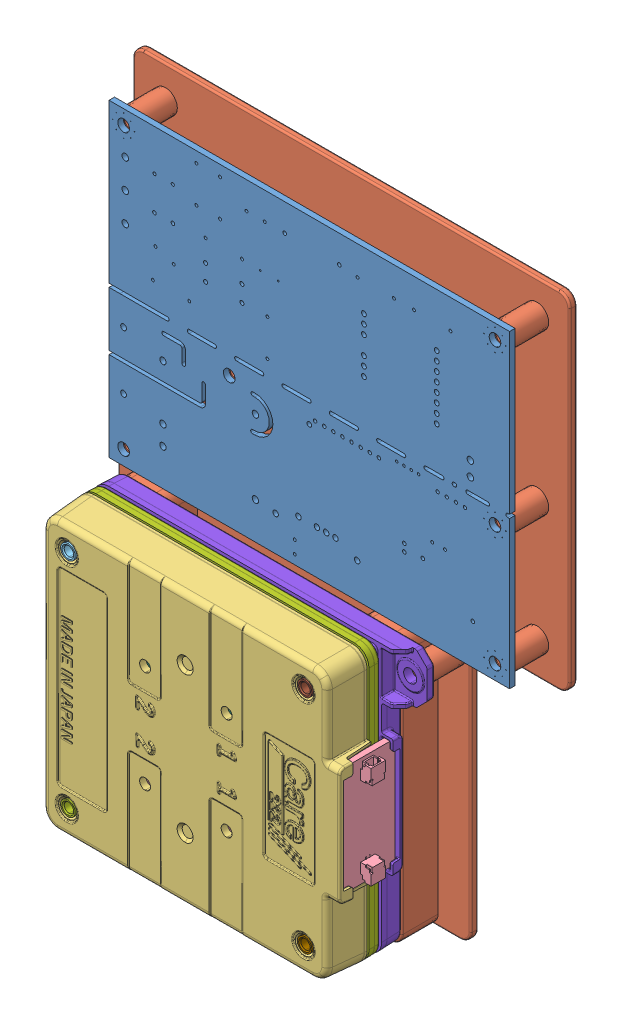
SolidWorks assembly osluv_test_assembly, configuration Default. Lengths in mm.
Overall size (124.12 167.88 32.3).
38 component instances, 33 part files, 8 mates.
Components (placement in the parent):
- osluv_pcb-1: osluv_pcb [Default] at (-161.3043 106.25 19.6144) size (110 85 1.51)
- test_fixture-1: test_fixture [Default] at (-161.3043 106.25 19.6144) x (-1 0 0) z (0 0 -1) size (124.12 167.88 12)
- emitter-1: emitter [Default] at (-120.388 -50.4736 -52.2117) x (0 -1 0) z (0 0 1) size (75 97 26.91)
  - emitter.step-1: emitter.step [Default] at origin size (75 97 26.91)
    - DRW1103739_UXFL70-222B4-UIA-Z1.STEP.step-1: DRW1103739_UXFL70-222B4-UIA-Z1.STEP.step [Default] at (-18.8418 87.9656 71.8261) size (75 97 26.91)
      - Z01_DRW1103184_LampCaseA.STEP.step-1: Z01_DRW1103184_LampCaseA.STEP.step [Default] at (0 3.0667 9.49) x (1 0 0) z (0 -1 0) size (75 10.8 82.07)
        - Z01_DRW1103184_LampCaseA-Part-1.STEP.step-1: Z01_DRW1103184_LampCaseA-Part-1.STEP.step [Default] at origin size (75 10.8 82.07)
        - Z01_DRW1103184_LampCaseA-Part-2.STEP.step-1: Z01_DRW1103184_LampCaseA-Part-2.STEP.step [Default] at origin size (4.3 4 4.3)
        - Z01_DRW1103184_LampCaseA-Part-3.STEP.step-1: Z01_DRW1103184_LampCaseA-Part-3.STEP.step [Default] at origin size (4.3 4 4.3)
        - Z01_DRW1103184_LampCaseA-Part-4.STEP.step-1: Z01_DRW1103184_LampCaseA-Part-4.STEP.step [Default] at origin size (4.3 4 4.3)
        - Z01_DRW1103184_LampCaseA-Part-5.STEP.step-1: Z01_DRW1103184_LampCaseA-Part-5.STEP.step [Default] at origin size (4.3 4 4.3)
        - Z01_DRW1103184_LampCaseA-Part-6.STEP.step-1: Z01_DRW1103184_LampCaseA-Part-6.STEP.step [Default] at origin size (4.3 4 4.3)
        - Z01_DRW1103184_LampCaseA-Part-7.STEP.step-1: Z01_DRW1103184_LampCaseA-Part-7.STEP.step [Default] at origin size (4.3 4 4.3)
        - Z01_DRW1103184_LampCaseA-Part-8.STEP.step-1: Z01_DRW1103184_LampCaseA-Part-8.STEP.step [Default] at origin size (4.3 4 4.3)
        - Z01_DRW1103184_LampCaseA-Part-9.STEP.step-1: Z01_DRW1103184_LampCaseA-Part-9.STEP.step [Default] at origin size (4.3 4 4.3)
      - Z14__[_q__X.STEP.step-1: Z14__[_q__X.STEP.step [Default] at (3.6282 -61.45 19.8) size (67.45 43.9 7.01)
        - Z14__[_q__X-Part-1.STEP.step-1: Z14__[_q__X-Part-1.STEP.step [Default] at origin size (67.45 33.11 7.01) (hidden)
        - Z14__[_q__X-Part-2.STEP.step-1: Z14__[_q__X-Part-2.STEP.step [Default] at origin size (65 14.5 3) (hidden)
        - Z14__[_q__X-Part-3.STEP.step-1: Z14__[_q__X-Part-3.STEP.step [Default] at origin size (65 14.5 3) (hidden)
      - Z07_DRW1100980-01______70_~52.STEP.step-1: Z07_DRW1100980-01______70_~52.STEP.step [Default] at (4.525 -65.5 1.8) x (1 0 0) z (0 0 1) size (70 52 0.5)
      - Z10_222nm____.STEP.step-1: Z10_222nm____.STEP.step [Default] at (58.5 -67.1323 10) x (0 1 0) z (0 0 -1) size (68 6 6)
      - Z10_222nm____-1.STEP.step-1: Z10_222nm____-1.STEP.step [Default] at (44.5 -67.1323 10) x (0 1 0) z (0 0 -1) size (68 6 6)
      - Z10_222nm____-2.STEP.step-1: Z10_222nm____-2.STEP.step [Default] at (30.5 -67.1323 10) x (0 1 0) z (0 0 -1) size (68 6 6)
      - Z10_222nm____-3.STEP.step-1: Z10_222nm____-3.STEP.step [Default] at (16.5 -67.1323 10) x (0 1 0) z (0 0 -1) size (68 6 6)
      - Z11_222nmUV-BP____i.STEP.step-1: Z11_222nmUV-BP____i.STEP.step [Default] at (70.5 -13.5 2.3) x (-1 0 0) z (0 0 1) size (70 52 1)
      - Z08_W___(P4___a)__________M2.6_~12.STEP.step-1: Z08_W___(P4___a)__________M2.6_~12.STEP.step [Default] at (7 -72 0.8139) x (0 0 1) z (0 -1 0) size (13.67 5 5)
      - Z08_W___(P4___a)__________M2.6_~12-1.STEP.step-1: Z08_W___(P4___a)__________M2.6_~12-1.STEP.step [Default] at (68 -72 0.8139) x (0 0 1) z (0 -1 0) size (13.67 5 5)
      - Z08_W___(P4___a)__________M2.6_~12-2.STEP.step-1: Z08_W___(P4___a)__________M2.6_~12-2.STEP.step [Default] at (68 -7 0.8139) x (0 0 1) z (0 -1 0) size (13.67 5 5)
      - Z08_W___(P4___a)__________M2.6_~12-3.STEP.step-1: Z08_W___(P4___a)__________M2.6_~12-3.STEP.step [Default] at (7 -7 0.8139) x (0 0 1) z (0 -1 0) size (13.67 5 5)
      - Z12_LED____.STEP.step-1: Z12_LED____.STEP.step [Default] at (22.4997 -0.9256 18.6001) x (1 0 0.000001) z (0 1 0) size (30 15 5.81)
      - Z07_DRW1100980-01______70_~52-1.STEP.step-1: Z07_DRW1100980-01______70_~52-1.STEP.step [Default] at (4.525 -65.5 3.3) x (1 0 0) z (0 0 1) size (70 52 0.5)
      - Z13_LED_____h_~__.STEP.step-1: Z13_LED_____h_~__.STEP.step [Default] at (41.5 -2.15 10.5) x (0 0 1) z (0 -1 0) size (8 8 1)
      - Z02_DRW1103185_LampCaseB.STEP.step-1: Z02_DRW1103185_LampCaseB.STEP.step [Default] at (-151.9677 -5.0437 3.4157) size (75 79 12.5)
      - Z03_DRW1103186_LampCaseC.STEP.step-1: Z03_DRW1103186_LampCaseC.STEP.step [Default] at (0 -88 0) size (75 97 6.11)
      - Z08_W___(P4___a)__________M2.6_~12-4.STEP.step-1: Z08_W___(P4___a)__________M2.6_~12-4.STEP.step [Default] at (51.5 -28.3 26.4861) x (0 0 -1) z (0 -1 0) size (13.67 5 5) (hidden)
      - Z08_W___(P4___a)__________M2.6_~12-5.STEP.step-1: Z08_W___(P4___a)__________M2.6_~12-5.STEP.step [Default] at (23.5 -28.3 26.4861) x (0 0 -1) z (0 -1 0) size (13.67 5 5) (hidden)
      - Z08_W___(P4___a)__________M2.6_~12-6.STEP.step-1: Z08_W___(P4___a)__________M2.6_~12-6.STEP.step [Default] at (23.5 -50.7 26.4861) x (0 0 -1) z (0 1 0) size (13.67 5 5) (hidden)
      - Z08_W___(P4___a)__________M2.6_~12-7.STEP.step-1: Z08_W___(P4___a)__________M2.6_~12-7.STEP.step [Default] at (51.5 -50.7 26.4861) x (0 0 -1) z (0 1 0) size (13.67 5 5) (hidden)
Mates (geometry in assembly coordinates):
- InPlace1: in place: plane of osluv_pcb-1 through (-161.3043 106.25 19.6144) normal (0 0 -1); plane of ? through (0 0 19.6144) normal (0 0 -1); moOrthogonalPlaneRef_w of osluv_pcb-1 through (-161.3043 106.25 19.6144) normal (0 0 -1); plane of ? through (0 0 19.6144) normal (0 1 0); plane of osluv_pcb-1 through (-161.3043 106.25 19.6144) normal (0 0 -1); plane of ? through (0 0 19.6144) normal (-1 0 0); plane of osluv_pcb-1 through (-161.3043 106.25 19.6144) normal (0 0 -1); unknown of test_fixture-1
- Coincident1: coincident aligned: plane of osluv_pcb-1; plane of test_fixture-1
- Coincident2: coincident aligned: moOrthogonalPlaneRef_w of osluv_pcb-1 through (-161.3043 106.25 19.6144) normal (0 1 0); plane of test_fixture-1 through (-161.3043 106.25 19.6144) normal (0 1 0)
- Coincident3: coincident anti-aligned: moOrthogonalPlaneRef_w of osluv_pcb-1 through (-161.3043 106.25 19.6144) normal (1 0 0); plane of test_fixture-1 through (-161.3043 106.25 19.6144) normal (-1 0 0)
- Coincident6: coincident aligned: plane of osluv_pcb-1 through (-161.3043 106.25 19.6144) normal (0 0 -1); plane of emitter-1/emitter.step-1/DRW1103739_UXFL70-222B4-UIA-Z1.STEP.step-1/Z03_DRW1103186_LampCaseC.STEP.step-1 through (-32.4224 -31.6318 19.6144) normal (0 0 -1)
- Parallel2: parallel: plane of osluv_pcb-1 through (-1.3043 -28.75 19.6144) normal (0 -1 0); line of emitter-1/emitter.step-1/DRW1103739_UXFL70-222B4-UIA-Z1.STEP.step-1/Z03_DRW1103186_LampCaseC.STEP.step-1 through (-26.8791 -31.75 20.1013) axis (-1 0 0)
- Coincident7: coincident: plane of osluv_pcb-1 through (-111.3043 -28.75 19.6144) normal (-1 0 0); line of emitter-1/emitter.step-1/DRW1103739_UXFL70-222B4-UIA-Z1.STEP.step-1/Z03_DRW1103186_LampCaseC.STEP.step-1 through (-111.3043 -35.7486 20.1013) axis (0 -1 0)
- Distance1: distance = 3 mm: plane of osluv_pcb-1 through (-1.3043 -28.75 19.6144) normal (0 -1 0); line of emitter-1/emitter.step-1/DRW1103739_UXFL70-222B4-UIA-Z1.STEP.step-1/Z03_DRW1103186_LampCaseC.STEP.step-1 through (-26.8791 -31.75 20.1013) axis (-1 0 0)
